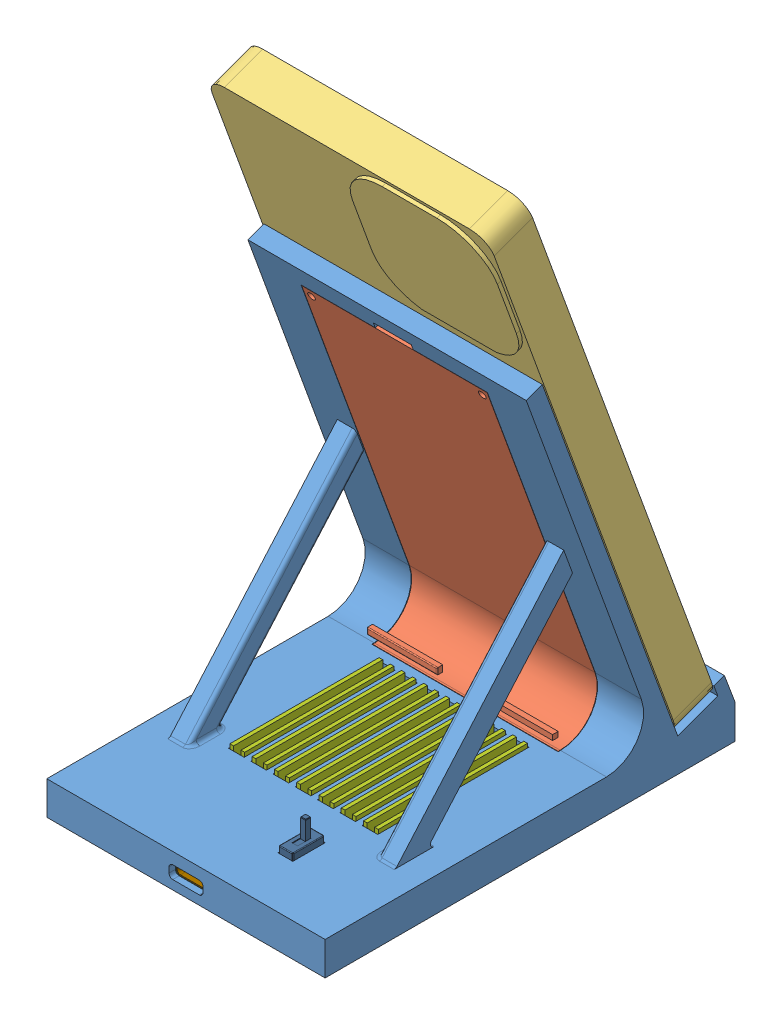
SolidWorks assembly IP支架装配体, configuration 默认. Lengths in mm.
Overall size (76 154.66 111.5).
31 component instances, 16 part files, 22 mates.
Components (placement in the parent):
- IP支架-1: IP支架 [默认] at (-19.3867 -35.6954 110) size (75 109.24 110.5)
- IP线圈支架零件-1: IP线圈支架零件 [默认] at (-19.3867 -31.7451 120.1792) x (0 0 -1) z (1 0 0) size (32.67 97.3 50)
- IP手机-1: IP手机 [默认] at (-19.3867 44.2514 95.8225) x (1 0 0) z (0 0.939693 0.34202) size (76 12 151)
- 充电线圈-1: 充电线圈 [默认] at (-19.3867 43.6338 97.6197) x (1 0 0) z (0 -0.939693 -0.34202) size (43 1.52 55.03)
- 充电零件板-1: 充电零件板 [默认] at (-19.3867 -30.6954 114.2678) x (1 0 0) z (0 0 -1) size (21 2 28)
- IP底板-1: IP底板 [默认] at (-35.435 -35.6954 107.1856) x (0 0 -1) z (1 0 0) size (102.06 5.8 64.8)
- 散热器-1: 散热器 [默认] at (-19.3867 -30.6954 113.06) size (40 5 40.2)
- TypeC电路板-2: TypeC电路板 [默认] at (-41.3838 -28.6954 166.4715) x (0 0 -1) z (0 -1 0) size (30 34.97 13.16)
  - TypeC电路板.STEP-1: TypeC电路板.STEP [默认] at origin size (30 34.97 13.16)
    - TypeC______.STEP.STEP-1: TypeC______.STEP.STEP [默认] at origin size (30 34.97 13.16)
      - 5v06-R1.STEP.STEP-1: 5v06-R1.STEP.STEP [默认] at (25.0953 30.8357 1.2) x (-1 0 0) z (0 0 1) size (2 1.3 0.61)
        - R0805.STEP.STEP-1: R0805.STEP.STEP [默认] at origin size (2 1.3 0.61)
          - COMPOUND.STEP.STEP-1: COMPOUND.STEP.STEP [默认] at origin size (2 1.3 0.61)
      - 5v06-USB1.STEP.STEP-1: 5v06-USB1.STEP.STEP [默认] at (8.1992 21.9972 1.2) x (0 -1 0) z (0 0 1) size (8.95 7.58 4.16)
        - USB-C-SMD_TYPE-C-6PIN-2MD-073.STEP.STEP-1: USB-C-SMD_TYPE-C-6PIN-2MD-073.STEP.STEP [默认] at origin size (8.95 7.58 4.16)
          - COMPOUND-1.STEP.STEP-1: COMPOUND-1.STEP.STEP [默认] at origin size (8.95 7.58 4.16)
      - 5v06-U2.STEP.STEP-1: 5v06-U2.STEP.STEP [默认] at (19.685 34.9251 0) x (-1 0 0) z (0 0 -1) size (8.51 3.81 11.5)
        - SW-TH_DEALON_SS-12D01-GX.STEP.STEP-1: SW-TH_DEALON_SS-12D01-GX.STEP.STEP [默认] at origin size (8.51 3.81 11.5)
          - COMPOUND-2.STEP.STEP-1: COMPOUND-2.STEP.STEP [默认] at origin size (8.51 3.81 11.5)
      - 5v06-C1.STEP.STEP-1: 5v06-C1.STEP.STEP [默认] at (18.2118 28.8799 1.2) size (3.2 2.52 0.9)
        - C1210.STEP.STEP-1: C1210.STEP.STEP [默认] at origin size (3.2 2.52 0.9)
          - SOLID-3.STEP.STEP-1: SOLID-3.STEP.STEP [默认] at origin size (3.2 2.52 0.9)
      - 5v06-C2.STEP.STEP-1: 5v06-C2.STEP.STEP [默认] at (24.13 13.843 1.2) x (0 1 0) z (0 0 1) size (1.6 0.8 0.8)
        - C0603.STEP.STEP-1: C0603.STEP.STEP [默认] at origin size (1.6 0.8 0.8)
          - SOLID-4.STEP.STEP-1: SOLID-4.STEP.STEP [默认] at origin size (1.6 0.8 0.8)
      - 5v06-U4.STEP.STEP-1: 5v06-U4.STEP.STEP [默认] at (18.386 14.645 1.2) size (4.1 4.3 1.61)
        - SOT-89-3_L4.5-W2.5-P1.50-LS4.2-BR.STEP.STEP-1: SOT-89-3_L4.5-W2.5-P1.50-LS4.2-BR.STEP.STEP [默认] at origin size (4.1 4.3 1.61)
          - SOLID-5.STEP.STEP-1: SOLID-5.STEP.STEP [默认] at origin size (4.1 4.3 1.61)
      - Board.STEP.STEP-1: Board.STEP.STEP [默认] at origin size (29.97 34.97 1.2)
- Led5mmRojo_.step-1: Led5mmRojo_.step [默认] at (-19.3867 -31.1954 79) x (0 0 -1) z (1 0 0) size (25.5 5.8 5.4)
- 配重块-1: 配重块 [默认] at (-19.3867 -34.1954 112.4387) x (0 0 1) z (-1 0 0) size (92 1.6 50)
Mates (geometry in assembly coordinates):
- 重合1: coincident anti-aligned: plane of IP支架-1 through (126.3422 73.5456 106.4847) normal (0 0.34202 -0.939693); plane of IP手机-1 through (-19.3867 44.2514 95.8225) normal (0 -0.34202 0.939693)
- 宽度1: width aligned: plane of IP支架-1 through (18.1133 -26.6954 165) normal (1 0 0); plane of IP支架-1 through (-56.8867 -26.6954 165) normal (-1 0 0); plane of IP手机-1 through (18.6133 -22.9332 59.6634) normal (1 0 0); plane of IP手机-1 through (-57.3867 -22.9332 59.6634) normal (-1 0 0)
- 重合8: coincident anti-aligned: plane of IP线圈支架零件-1 through (-19.3867 43.1207 99.0292) normal (0 0.34202 -0.939693); plane of 充电线圈-1 through (-19.3867 43.1207 99.0292) normal (0 -0.34202 0.939693)
- 同心1: concentric aligned: cylinder of IP线圈支架零件-1 through (-19.3867 43.1207 99.0292) axis (0 0.34202 -0.939693) radius 22; cylinder of 充电线圈-1 through (-19.3867 43.1207 99.0292) axis (0 0.34202 -0.939693) radius 21.5
- 重合15: coincident aligned: plane of IP线圈支架零件-1 through (-19.3867 -31.7451 120.1792) normal (1 0 0); plane of 充电线圈-1 through (-19.3867 43.6338 97.6197) normal (1 0 0)
- 宽度8: width aligned: plane of IP支架-1 through (18.1133 -26.6954 165) normal (1 0 0); plane of 散热器-1 through (-56.8867 -26.6954 165) normal (-1 0 0); plane of IP支架-1 through (0.6133 -28.6954 92.96) normal (1 0 0); plane of 散热器-1 through (-39.3867 -28.6954 92.96) normal (-1 0 0)
- 距离4: distance = 31.84 mm aligned: plane of 散热器-1 through (-39.3867 -28.6954 133.16) normal (0 0 1); plane of IP支架-1 through (-56.8867 -26.6954 165) normal (0 0 1)
- 重合43: coincident anti-aligned: plane of 充电零件板-1 through (-21.3867 -30.6954 108.6428) normal (0 1 0); plane of 散热器-1 through (-19.3867 -30.6954 113.06) normal (0 -1 0)
- 宽度9: width aligned: plane of 散热器-1 through (-39.3867 -28.6954 92.96) normal (-1 0 0); plane of 散热器-1 through (0.6133 -28.6954 92.96) normal (1 0 0); plane of 充电零件板-1 through (-29.8867 -32.6954 125.2678) normal (-1 0 0); plane of 充电零件板-1 through (-8.8867 -32.6954 125.2678) normal (1 0 0)
- 重合44: coincident aligned: plane of IP支架-1 through (-19.3867 -35.6954 110) normal (0 -1 0); plane of IP底板-1 through (-35.435 -35.6954 107.1856) normal (0 -1 0)
- 宽度11: width anti-aligned: plane of IP支架-1 through (-400019.3867 -35.6964 159) normal (0 0 -1); plane of IP底板-1 through (-400019.3867 -35.6964 61) normal (0 0 1); plane of IP支架-1 through (-51.7867 -34.1954 158.9) normal (0 0 1); plane of IP底板-1 through (-51.7867 -34.1954 61.1) normal (0 0 -1)
- 重合52: coincident anti-aligned: plane of IP支架-1 through (-79.7288 -26.6954 70) normal (0 0.939693 0.34202); plane of IP手机-1 through (-57.3867 -22.9332 59.6634) normal (0 -0.939693 -0.34202)
- 距离9: distance = 0.1 mm anti-aligned: plane of TypeC电路板-2/TypeC电路板.STEP-1/TypeC______.STEP.STEP-1/Board.STEP.STEP-1 through (-1.8994 -28.6954 133.26) normal (0 0 -1); plane of 散热器-1 through (-39.3867 -28.6954 133.16) normal (0 0 1)
- 宽度15: width aligned: plane of IP支架-1 through (13.1133 -35.6964 291687.6203) normal (-1 0 0); plane of IP支架-1 through (-51.8867 -35.6964 291687.6203) normal (1 0 0); plane of TypeC电路板-2/TypeC电路板.STEP-1/TypeC______.STEP.STEP-1/Board.STEP.STEP-1 through (-36.874 -28.6954 133.26) normal (-1 0 0); plane of TypeC电路板-2/TypeC电路板.STEP-1/TypeC______.STEP.STEP-1/Board.STEP.STEP-1 through (-1.8994 -28.6954 155.7346) normal (1 0 0)
- 宽度16: width: plane of IP支架-1 through (-19.3867 -35.6954 110) normal (0 -1 0); plane of Led5mmRojo_.step-1 through (-19.3867 -26.6954 110) normal (0 1 0); cylinder of IP支架-1 through (-19.3867 -31.1954 61) axis (0 0 -1) radius 2.5
- 宽度17: width: plane of IP支架-1 through (18.1133 -26.6954 165) normal (1 0 0); plane of Led5mmRojo_.step-1 through (-56.8867 -26.6954 165) normal (-1 0 0); cylinder of IP支架-1 through (-19.3867 -31.1954 61) axis (0 0 -1) radius 2.5
- 平行1: parallel aligned: plane of IP支架-1 through (-19.3867 -35.6954 110) normal (0 -1 0); plane of Led5mmRojo_.step-1 through (-18.3667 -31.4454 62) normal (0 -1 0)
- 重合55: coincident anti-aligned: plane of IP支架-1 through (-400019.3867 -35.6964 61) normal (0 0 1); plane of Led5mmRojo_.step-1 through (-19.1867 -31.1954 61) normal (0 0 -1)
- 重合56: coincident anti-aligned: plane of IP支架-1 through (-19.3867 -28.6954 110) normal (0 -1 0); plane of TypeC电路板-2/TypeC电路板.STEP-1/TypeC______.STEP.STEP-1/Board.STEP.STEP-1 through (-19.3867 -28.6954 146.9186) normal (0 1 0)
- 重合57: coincident anti-aligned: plane of IP支架-1 through (-19.3867 -28.6954 110) normal (0 -1 0); plane of 散热器-1 through (-19.3867 -28.6954 113.06) normal (0 1 0)
- 重合59: coincident anti-aligned: plane of IP底板-1 through (-35.435 -34.1954 107.1856) normal (0 1 0); plane of 配重块-1 through (-19.3867 -34.1954 112.4387) normal (0 -1 0)
- 宽度18: width aligned: plane of IP底板-1 through (-51.7867 -34.1954 158.9) normal (-1 0 0); plane of 配重块-1 through (13.0133 -34.1954 158.9) normal (1 0 0); plane of IP底板-1 through (-44.3867 -32.5954 66.4387) normal (-1 0 0); plane of 配重块-1 through (5.6133 -32.5954 66.4387) normal (1 0 0)
